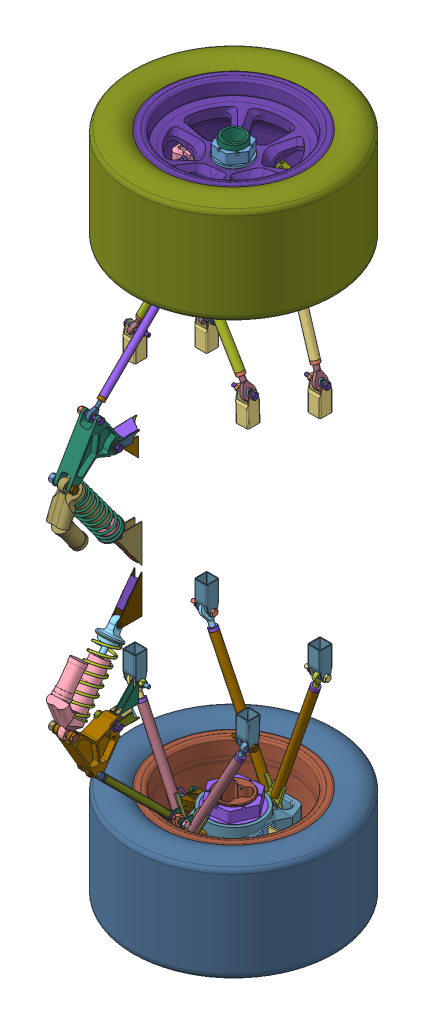
SolidWorks assembly UN-A1001-AB-Rear Unsprung Assembly, configuration Default. Lengths in mm. (continued)
Components (placement in the parent): (continued)
- SP-A0200-AH-Rear Axle AssemblyMirror-2: SP-A0200-AH-Rear Axle AssemblyMirror [Default] x (1 0 0) z (0 0 -1) size (274.88 563.57 484.64)
  - SP-AA-Rear Lower A-ArmMirror^SP-A0200-AH-Rear Axle Assembly-1: SP-AA-Rear Lower A-ArmMirror^SP-A0200-AH-Rear Axle Assembly [Default] at (0 -0.399 -0.6588) x (1 0 0) z (0 -0.002866 0.999996) size (222.76 290.57 36.42)
    - SP-Lower Apex RearMirror-1: SP-Lower Apex RearMirror [Default] at (-792.4265 549.6462 -121.5417) x (-0.932505 -0.360479 -0.022123) z (0 0.061256 -0.998122) size (54.94 63.8 9.53)
    - MirrorFS-MALE ROD END UNF-3A, 0.3125x24-0.25D (XAM-4)1Mirror-1: MirrorFS-MALE ROD END UNF-3A, 0.3125x24-0.25D (XAM-4)1Mirror [Default] at (-906.7265 255.0788 -139.6197) x (0.932505 -0.360479 -0.022123) z (0.361157 0.930754 0.057121)
    - MirrorFS-MALE ROD END UNF-3A, 0.3125x24-0.25D (XAM-4)1Mirror-2: MirrorFS-MALE ROD END UNF-3A, 0.3125x24-0.25D (XAM-4)1Mirror [Default] at (-678.1265 255.0788 -139.6197) x (0.932505 0.360479 0.022123) z (-0.361157 0.930754 0.057121)
    - SP-10003-AB-Threaded InsertMirror-1: SP-10003-AB-Threaded InsertMirror [A-Arm] at (-890.6731 296.4508 -137.0806) x (0.932505 -0.360479 -0.022123) z (0.361157 0.930754 0.057121) size (15.88 15.88 15.88)
    - SP-10003-AB-Threaded InsertMirror-2: SP-10003-AB-Threaded InsertMirror [A-Arm] at (-694.18 296.4508 -137.0806) x (0.932505 0.360479 0.022123) z (-0.361157 0.930754 0.057121) size (15.88 15.88 15.88)
    - SP-Rear Lower A-Arm TubeMirror-1: SP-Rear Lower A-Arm TubeMirror [Default] at (-838.6322 430.5677 -128.8497) x (-0.361157 -0.930754 -0.057121) z (0 0.061256 -0.998122) size (257.84 15.88 15.88)
    - SP-Rear Lower A-Arm TubeMirror-2: SP-Rear Lower A-Arm TubeMirror [Default] at (-746.2209 430.5677 -128.8497) x (0.361157 -0.930754 -0.057121) z (0 -0.061256 0.998122) size (257.84 15.88 15.88)
    - FS-HIGH MISALIGN SPHERICAL BEARING, 0.375-0.906D (3072-6G)Mirror-1: Assem24 [Default] at (-792.4265 549.6462 -121.5417) x (-0.932505 0.360479 0.022123) z (0.361157 0.930754 0.057121) size (26.46 21.71 26.13)
      - RaceMirror^FS-HIGH MISALIGN SPHERICAL BEARING, 0.375-0.906D (3072-6G)-1: Part65 [Default] at origin size (23.01 8.76 23.01)
      - BallMirror^FS-HIGH MISALIGN SPHERICAL BEARING, 0.375-0.906D (3072-6G)-1: Part66 [Default] x (0.359576 -0.008176 -0.93308) z (0.932238 0.046516 0.358844) size (19.84 20.65 19.84)
  - SP-AA-Rear Upper A-ArmMirror^SP-A0200-AH-Rear Axle Assembly-1: SP-AA-Rear Upper A-ArmMirror^SP-A0200-AH-Rear Axle Assembly [Default] at (-38.1 -1.9308 -1.9372) x (1 0 0) z (0 -0.00685 0.999977) size (216 215.55 29.43)
    - SP-Upper Apex RearMirror-1: SP-Upper Apex RearMirror [Default] at (-755.8405 523.8827 -293.8505) x (0.884705 -0.465567 0.023329) z (0 0.050046 0.998747) size (76.45 83.12 9.53)
    - MirrorFS-MALE ROD END UNF-3A, 0.3125x24-0.25D (XAM-4)1Mirror-1: MirrorFS-MALE ROD END UNF-3A, 0.3125x24-0.25D (XAM-4)1Mirror [Default] at (-870.1405 307.2255 -282.9942) x (0.884705 -0.465567 0.023329) z (0.466151 0.883596 -0.044276)
    - MirrorFS-MALE ROD END UNF-3A, 0.3125x24-0.25D (XAM-4)1Mirror-2: MirrorFS-MALE ROD END UNF-3A, 0.3125x24-0.25D (XAM-4)1Mirror [Default] at (-641.5405 307.2255 -282.9942) x (0.884705 0.465567 -0.023329) z (-0.466151 0.883596 -0.044276)
    - SP-10003-AB-Threaded InsertMirror-1: SP-10003-AB-Threaded InsertMirror [A-Arm] at (-849.4201 346.5014 -284.9623) x (0.884705 -0.465567 0.023329) z (0.466151 0.883596 -0.044276) size (15.88 15.88 15.88)
    - SP-10003-AB-Threaded InsertMirror-2: SP-10003-AB-Threaded InsertMirror [A-Arm] at (-662.261 346.5014 -284.9623) x (0.884705 0.465567 -0.023329) z (-0.466151 0.883596 -0.044276) size (15.88 15.88 15.88)
    - SP-Rear Upper A-Arm TubeMirror-1: SP-Rear Upper A-Arm TubeMirror [Default] at (-812.9905 415.5541 -288.4224) x (0.466151 0.883596 -0.044276) z (-0.884705 0.465567 -0.023329) size (186.28 15.88 15.88)
    - SP-Rear Upper A-Arm TubeMirror-2: SP-Rear Upper A-Arm TubeMirror [Default] at (-698.6905 415.5541 -288.4224) x (-0.466151 0.883596 -0.044276) z (-0.884705 -0.465567 0.023329) size (186.28 15.88 15.88)
    - FS-HIGH MISALIGN SPHERICAL BEARING, 0.375-0.906D (3072-6G)Mirror-1: Assem28 [Default] at (-755.8405 523.8827 -293.8505) x (0.884705 -0.465567 0.023329) z (0.466151 0.883596 -0.044276) size (26.46 21.71 26.13)
      - RaceMirror^FS-HIGH MISALIGN SPHERICAL BEARING, 0.375-0.906D (3072-6G)-1: Part69 [Default] at origin size (23.01 8.76 23.01)
      - BallMirror^FS-HIGH MISALIGN SPHERICAL BEARING, 0.375-0.906D (3072-6G)-1: Part70 [Default] x (0.359576 -0.008176 -0.93308) z (0.932238 0.046516 0.358844) size (19.84 20.65 19.84)
  - Assem8Mirror^SP-A0200-AH-Rear Axle Assembly-1: Assem8Mirror^SP-A0200-AH-Rear Axle Assembly [Default] at (-1592.9214 814.7933 -712.2762) x (-0.999891 -0.01037 -0.010464) z (-0.012143 0.982316 0.186836) size (17.98 166.51 230.13)
    - Part2Mirror^Assem8_SP-A0200-AH-Rear Axle Assembly-1: Part2Mirror^Assem8_SP-A0200-AH-Rear Axle Assembly [Default] at origin size (15.39 113.92 157.78)
    - SP-10003-AC-Threaded InsertMirror-1: SP-10003-AC-Threaded InsertMirror [AM-4 Rod End Thread] at (-799.064 427.6015 -294.0449) x (-0.999891 -0.008342 -0.012143) z (0.014733 -0.566176 -0.824153) size (12.7 12.7 15.88)
    - SP-10003-AC-Threaded InsertMirror-2: SP-10003-AC-Threaded InsertMirror [AM-4 Rod End Thread] at (-796.6527 334.9355 -428.9338) x (-0.999891 -0.008342 -0.012143) z (-0.014733 0.566176 0.824153) size (12.7 12.7 15.88)
    - FS-MALE ROD END UNF-3A, 0.25x28-0.25D (AM-4)Mirror-1: Assem30 [Default] at (-796.0446 311.5665 -462.9507) x (0 -0.824242 0.566238) z (0.014733 -0.566176 -0.824153) size (19.32 14.06 49.44)
      - BodyMirror^FS-MALE ROD END UNF-3A, 0.25x28-0.25D (AM-4)-1: Part73 [Default] at origin size (19.32 7.2 49.44)
      - BallMirror^FS-MALE ROD END UNF-3A, 0.25x28-0.25D (AM-4)-1: Part74 [Default] x (0.09633 0.218783 -0.971007) z (0.984027 -0.167661 0.059845) size (12.7 9.53 12.7)
    - FS-MALE ROD END UNF-3A, 0.25x28-0.25D (AM-4)Mirror-2: Assem31 [Default] at (-799.6721 450.9704 -260.028) x (0 -0.824242 0.566238) z (-0.014733 0.566176 0.824153) size (19.32 14.06 49.44)
      - BodyMirror^FS-MALE ROD END UNF-3A, 0.25x28-0.25D (AM-4)-1: Part75 [Default] at origin size (19.32 7.2 49.44)
      - BallMirror^FS-MALE ROD END UNF-3A, 0.25x28-0.25D (AM-4)-1: Part76 [Default] x (0.09633 0.218783 -0.971007) z (0.984027 -0.167661 0.059845) size (12.7 9.53 12.7)
  - SP-A0105-AC-Ohlin TTX25 MKII, 200mmMirror-1: SP-A0105-AC-Ohlin TTX25 MKII, 200mmMirror [Default] at (-793.9406 216.4917 -537.8809) x (-1 0 0) z (0 -0.803503 0.5953) size (48.39 85.02 197.6)
    - Shock BodyMirror^SP-A0105-AC-Ohlin TTX25 MKII, 200mm-1: Shock BodyMirror^SP-A0105-AC-Ohlin TTX25 MKII, 200mm [Default] at origin size (40.76 80 131.7)
    - HeadMirror^SP-A0105-AC-Ohlin TTX25 MKII, 200mm-1: HeadMirror^SP-A0105-AC-Ohlin TTX25 MKII, 200mm [Default] at (0 0 174.6) size (46 46 119)
    - BallMirror^SP-A0105-AC-Ohlin TTX25 MKII, 200mm-1: BallMirror^SP-A0105-AC-Ohlin TTX25 MKII, 200mm [Default] at (0 0 174.6) x (-0.011681 0.107343 -0.994153) z (-0.993776 -0.111394 -0.000351) size (15 15 8)
    - BallMirror^SP-A0105-AC-Ohlin TTX25 MKII, 200mm-2: BallMirror^SP-A0105-AC-Ohlin TTX25 MKII, 200mm [Default] x (0.079523 -0.862756 0.499328) z (-0.965926 0.057074 0.252448) size (15 15 8)
    - SP-#####-AB-SpringMirror-1: SP-#####-AB-SpringMirror [Default] at (0 0 151.1) size (48.39 49.05 127.97)
  - FS-BALL BEARING, 0.25ID-0.75OD (60355K702)Mirror-1: Part81 [Default] at (-784.8125 243.84 -446.6415) x (0 -0.287121 -0.957894) z (1 0 0) size (19.05 19.05 7.14)
  - FS-BALL BEARING, 0.25ID-0.75OD (60355K702)Mirror-2: Part82 [Default] at (-803.0688 243.84 -446.6415) x (0 0.287121 0.957894) z (-1 0 0) size (19.05 19.05 7.14)
  - FS-CADMIUM PLATED C3 HEX, 0.25x28-1.65-0.469 (AN4-13A)Mirror-1: Part83 [Default] at (-796.8362 310.0391 -484.3789) x (-1 0 0) z (0 -0.868755 0.495242) size (46.28 12.9 11.18)
  - FS-ZINC YELLOW CHROMATE C10.9 HX, M8x1.25-40-22 (95327A569)Mirror-1: Part84 [Default] at (-795.4156 216.4917 -537.8809) x (-1 0 0) z (0 0.287121 0.957894) size (45.3 15.01 13)
  - FS-NYLOC FLHX C8, M8x1.25-11.1 (92461A400)Mirror-1: Part85 [Default] at (-820.9156 216.4917 -537.8809) x (0 0.868058 0.496463) z (1 0 0) size (17.9 17.9 11.1)
  - FS-NYLOC G8 HX, 0.25x28-0.3125 (90630A145)Mirror-1: Part86 [Default] at (-809.8156 310.0391 -484.3789) x (0 0.868058 0.496463) z (0 -0.496463 0.868058) size (11.11 7.94 12.83)
  - SP-C30066-AA-A-Arm Tab BoxMirror-1: SP-C30066-AA-A-Arm Tab BoxMirror [Default] at (-680.9758 289.7175 -282.8202) x (-0.029021 0.999579 0) z (0 0 -1) size (60.32 25.4 25.4)
  - SP-C30066-AA-A-Arm Tab BoxMirror-2: SP-C30066-AA-A-Arm Tab BoxMirror [Default] at (-908.2405 289.7636 -282.8202) x (0 1 0) z (0 0 -1) size (60.32 25.4 25.4)
  - SP-C30066-AA-A-Arm Tab BoxMirror-3: SP-C30066-AA-A-Arm Tab BoxMirror [Default] at (-678.1265 237.6164 -139.5469) x (0 1 0) z (0 0 1) size (60.32 25.4 25.4)
  - SP-C30066-AA-A-Arm Tab BoxMirror-4: SP-C30066-AA-A-Arm Tab BoxMirror [Default] at (-906.7265 237.6164 -139.5469) x (0 1 0) z (0 0 1) size (60.32 25.4 25.4)
  - MirrorSP-30063-AB-Pushrod TabMirror-1: MirrorSP-30063-AB-Pushrod TabMirror [Default] at (-782.0343 483.2134 -293.6084) x (1 0 0) z (0 -0.043203 -0.999066) size (1.59 15.88 23.81)
  - MirrorSP-30063-AB-Pushrod TabMirror-2: MirrorSP-30063-AB-Pushrod TabMirror [Default] at (-805.8468 483.2134 -293.6084) x (-1 0 0) z (0 -0.043203 -0.999066) size (1.59 15.88 23.81)
  - FS-NYLOC FLHX C8, M8x1.25-11.1 (92461A400)Mirror-2: Part89 [Default] at (-820.9156 243.84 -446.6415) x (0 0 1) z (1 0 0) size (17.9 17.9 11.1)
  - FS-CADMIUM PLATED C3 HEX, 0.25x28-1.65-0.469 (AN4-13A)Mirror-2: Part90 [Default] at (-796.8362 243.84 -446.6415) x (-1 0 0) z (0 -0.287121 -0.957894) size (46.28 12.9 11.18)
  - FS-CADMIUM PLATED C3 HEX, 0.25x28-1.65-0.469 (AN4-13A)Mirror-3: Part91 [Default] at (-687.5506 306.9965 -282.8202) x (-0.999579 -0.029021 0) z (0 0 -1) size (46.28 12.9 11.18)
  - FS-CADMIUM PLATED C3 HEX, 0.25x28-1.65-0.469 (AN4-13A)Mirror-4: Part92 [Default] at (-902.1699 307.2261 -282.8202) size (46.28 12.9 11.18)
  - FS-CADMIUM PLATED C3 HEX, 0.25x28-1.65-0.469 (AN4-13A)Mirror-5: Part93 [Default] at (-912.7971 255.0789 -139.5469) x (-1 0 0) z (0 0 -1) size (46.28 12.9 11.18)
  - FS-CADMIUM PLATED C3 HEX, 0.25x28-1.65-0.469 (AN4-13A)Mirror-6: Part94 [Default] at (-684.1971 255.0789 -139.5469) x (-1 0 0) z (0 0 -1) size (46.28 12.9 11.18)
  - FS-CADMIUM PLATED C3 HEX, 0.25x28-1.65-0.469 (AN4-13A)Mirror-7: Part95 [Default] at (-799.2174 482.5275 -309.4686) x (-1 0 0) z (0 0.609051 0.793131) size (46.28 12.9 11.18)
  - FS-NYLOC G8 HX, 0.25x28-0.3125 (90630A145)Mirror-2: Part96 [Default] at (-807.4343 482.5275 -309.4686) x (0 -0.043203 -0.999066) z (0 0.999066 -0.043203) size (11.11 7.94 12.83)
  - FS-NYLOC G8 HX, 0.25x28-0.3125 (90630A145)Mirror-3: Part97 [Default] at (-694.1772 306.8041 -282.8202) x (-0.029021 0.999579 0) z (0 0 1) size (11.11 7.94 12.83)
  - FS-NYLOC G8 HX, 0.25x28-0.3125 (90630A145)Mirror-4: Part98 [Default] at (-895.5405 307.2261 -282.8202) x (0 1 0) z (0 0 -1) size (11.11 7.94 12.83)
  - FS-NYLOC G8 HX, 0.25x28-0.3125 (90630A145)Mirror-5: Part99 [Default] at (-919.4265 255.0789 -139.5469) x (0 1 0) z (0 0 1) size (11.11 7.94 12.83)
  - FS-NYLOC G8 HX, 0.25x28-0.3125 (90630A145)Mirror-6: Part100 [Default] at (-690.8265 255.0789 -139.5469) x (0 -1 0) z (0 0 -1) size (11.11 7.94 12.83)
  - FS-ROD END RETAINING WASHER, 0.25-0.245 (NO PN)Mirror-1: Part101 [Default] at (-781.9073 482.5275 -309.4686) x (0 1 0) z (1 0 0) size (12.7 12.7 6.22)
  - FS-ROD END RETAINING WASHER, 0.25-0.245 (NO PN)Mirror-2: Part102 [Default] at (-805.9738 482.5275 -309.4686) x (0 0.978954 -0.204082) z (-1 0 0) size (12.7 12.7 6.22)
  - SP-A0200-Rear Inner Rocker GussetMirror-1: SP-A0200-Rear Inner Rocker GussetMirror [Default] at (-793.9406 234.6955 -425.4808) x (1 0 0) z (0 -0.052336 0.99863) size (26.99 1.59 48.67)
  - SP-A0200-Rear Long Rocker TabMirror-1: SP-A0200-Rear Long Rocker TabMirror [Rear] at (-807.4344 243.84 -446.6415) x (1 0 0) z (0 0.00621 -0.999981) size (1.59 19.05 73.11)
  - SP-A0200-Rear Outer Rocker GussetMirror-1: SP-A0200-Rear Outer Rocker GussetMirror [Default] at (-793.9406 251.3902 -418.9606) x (1 0 0) z (0 0.039929 0.999203) size (26.99 1.59 43.52)
  - SP-A0200-Rear Rocker Gusset SupportMirror-1: SP-A0200-Rear Rocker Gusset SupportMirror [Default] at (-800.2906 228.5949 -403.7833) x (0 0 -1) z (0 -1 0) size (38.05 1.59 40.09)
  - SP-A0200-Rear Short Rocker TabMirror-1: SP-A0200-Rear Short Rocker TabMirror [Rear] at (-780.4469 243.8408 -446.6212) x (1 0 0) z (0 0.00621 -0.999981) size (1.59 17.17 50.59)
  - SP-A0200-Rear Rocker Gusset SupportMirror-2: SP-A0200-Rear Rocker Gusset SupportMirror [Default] at (-789.8131 228.5949 -403.7833) x (0 0 -1) z (0 -1 0) size (38.05 1.59 40.09)
  - SP-A0200-Rear Shock GussetMirror-1: SP-A0200-Rear Shock GussetMirror [Default] at (-793.9406 34.3591 -413.4634) x (1 0 0) z (0 -0.809017 0.587785) size (14.29 1.59 50.8)
  - SP-A0200-Rear Shock TabMirror-1: SP-A0200-Rear Shock TabMirror [Rear] at (-786.7969 76.2 -433.9415) x (-1 0 0) z (0 0.809017 -0.587785) size (1.59 45.95 88.76)
  - SP-A0200-Rear Shock TabMirror-2: SP-A0200-Rear Shock TabMirror [Front] at (-801.0844 76.2 -433.9415) x (-1 0 0) z (0 0.809017 -0.587785) size (1.59 45.95 88.76)
  - FS-MALE ROD END UNJF-3A, 0.375x24-0.25D (HXAM-4T)Mirror-1: Assem33 [Default] at (-679.6405 307.2261 -282.8202) x (0 0.043203 0.999066) z (0.466151 -0.883879 0.038222) size (26.22 15.06 62.54)
    - BodyMirror^FS-MALE ROD END UNJF-3A, 0.375x24-0.25D (HXAM-4T)-1: Part110 [no_threads] at origin size (26.22 9.62 62.54)
    - BallMirror^FS-MALE ROD END UNJF-3A, 0.375x24-0.25D (HXAM-4T)-1: Part111 [Default] at origin size (15.06 15.06 15.06)
  - FS-MALE ROD END UNJF-3A, 0.375x24-0.25D (HXAM-4T)Mirror-2: Assem34 [Default] at (-908.2405 307.2261 -282.8202) x (0 -0.043203 -0.999066) z (-0.466151 -0.883879 0.038222) size (26.22 15.06 62.54)
    - BodyMirror^FS-MALE ROD END UNJF-3A, 0.375x24-0.25D (HXAM-4T)-1: Part112 [no_threads] at origin size (26.22 9.62 62.54)
    - BallMirror^FS-MALE ROD END UNJF-3A, 0.375x24-0.25D (HXAM-4T)-1: Part113 [Default] at origin size (15.06 15.06 15.06)
  - FS-MALE ROD END UNJF-3A, 0.375x24-0.25D (HXAM-4T)Mirror-3: Assem35 [Default] at (-906.7265 255.0789 -139.5469) x (0 0.064116 -0.997942) z (-0.361157 -0.930586 -0.059789) size (26.22 15.06 62.54)
    - BodyMirror^FS-MALE ROD END UNJF-3A, 0.375x24-0.25D (HXAM-4T)-1: Part114 [no_threads] at origin size (26.22 9.62 62.54)
    - BallMirror^FS-MALE ROD END UNJF-3A, 0.375x24-0.25D (HXAM-4T)-1: Part115 [Default] at origin size (15.06 15.06 15.06)
  - FS-MALE ROD END UNJF-3A, 0.375x24-0.25D (HXAM-4T)Mirror-4: Assem36 [Default] at (-678.1265 255.0789 -139.5469) x (0 -0.064116 0.997942) z (0.361157 -0.930586 -0.059789) size (26.22 15.06 62.54)
    - BodyMirror^FS-MALE ROD END UNJF-3A, 0.375x24-0.25D (HXAM-4T)-1: Part116 [no_threads] at origin size (26.22 9.62 62.54)
    - BallMirror^FS-MALE ROD END UNJF-3A, 0.375x24-0.25D (HXAM-4T)-1: Part117 [Default] at origin size (15.06 15.06 15.06)
  - SP-B0100-Rear RockerMirror-1: SP-B0100-Rear RockerMirror [Default] at (14.7593 458.8134 310.4211) x (0.993764 -0.111506 0.000215) z (0.085107 0.759728 0.644647) size (43.51 92.41 122.03)
- WT-A0100-XG-Corner AssemblyMirror-2: WT-A0100-XG-Corner AssemblyMirror [Default] x (1 0 0) z (0 0 -1) size (411.48 213.6 411.53)
  - WT-00202-AA-Hoosier R25B 16x7_5-10Mirror-1: WT-00202-AA-Hoosier R25B 16x7_5-10Mirror [Default] at (-793.1174 574.9879 -198.909) x (-1 0 0) z (0 1 0.000253) size (411.48 411.48 213.5)
  - WT-00201-AA-OZ Centerlock 10in WheelMirror-1: WT-00201-AA-OZ Centerlock 10in WheelMirror [Default] at (-793.1174 596.9879 -198.9034) x (-0.992442 0.000031 -0.122714) z (0 -1 -0.000253) size (288.79 288.79 189.86)
  - WT-10105-AA-Drive PinMirror-1: WT-10105-AA-Drive PinMirror [Default] at (-825.0424 596.994 -223.0032) x (-0.121576 0.000251 -0.992582) z (0.992582 0.000031 -0.121576) size (12.67 23.01 11.95)
  - WT-10102-AA-Centerlock NutMirror-1: WT-10102-AA-Centerlock NutMirror [Default] at (-793.1174 647.6073 -198.8906) x (-0.440541 -0.000227 0.897732) z (-0.897733 0.000111 -0.440541) size (66 31.75 66)
  - WT-XF-UprightMirror-1: WT-XF-UprightMirror [Default] at (-793.1174 537.8923 -198.9183) x (-0.999961 -0.000002 0.008824) z (0.008824 -0.000253 0.999961) size (134.42 50.23 211.08)
  - BR-A0102-AA-Caliper AssemblyMirror-1: BR-A0102-AA-Caliper AssemblyMirror [Default] at (-874.0145 570.8565 -194.5235) x (-0.069854 0.000252 -0.997557) z (0 1 0.000253) size (82.63 68.94 66.64)
    - cp3838-M08x1.25m_CP4477-110Mirror^BR-A0102-AA-Caliper Assembly-1: Part124 [Default] at (-13.37 19.3 -19.55) x (-0.999952 -0.009843 0) z (0 0 -1) size (13 13 46)
    - CP4226-102Mirror^BR-A0102-AA-Caliper Assembly-1: CP4226-102Mirror^BR-A0102-AA-Caliper Assembly [Default] x (-1 0 0) z (0 0 -1) size (63.87 47.42 31.57)
    - cp4226-104_CP4226-104Mirror^BR-A0102-AA-Caliper Assembly-1: cp4226-104_CP4226-104Mirror^BR-A0102-AA-Caliper Assembly [Default] at (0 23 31.9644) x (0 0 -1) z (1 0 0) size (61.35 20.1 3)
    - CP4226-101Mirror^BR-A0102-AA-Caliper Assembly-1: CP4226-101Mirror^BR-A0102-AA-Caliper Assembly [Default] at origin size (81.26 55.69 34.68)
    - cp3838-M08x1.25m_CP4477-110Mirror^BR-A0102-AA-Caliper Assembly-2: Part128 [Default] at (13.37 19.3 -19.55) x (-0.997666 -0.068288 0) z (0 0 -1) size (13 13 46)
    - cp3049-40a_CP4226-103Mirror^BR-A0102-AA-Caliper Assembly-1: cp3049-40a_CP4226-103Mirror^BR-A0102-AA-Caliper Assembly [Default] at (0 0 -10.305) x (-0.993137 0.116957 0) z (0 0 -1) size (25.2 25.2 14.87)
    - CP4469-101Mirror^BR-A0102-AA-Caliper Assembly-1: CP4469-101Mirror^BR-A0102-AA-Caliper Assembly [Default] at (42 -11.5 23.98) x (0 -0.520643 -0.853775) z (1 0 0) size (9.18 8.2 29.15)
    - cp3049-40a_CP4226-103Mirror^BR-A0102-AA-Caliper Assembly-2: cp3049-40a_CP4226-103Mirror^BR-A0102-AA-Caliper Assembly [Default] at (0 0 10.305) size (25.2 25.2 14.87)
    - Brake PadMirror^BR-A0102-AA-Caliper Assembly-1: Brake PadMirror^BR-A0102-AA-Caliper Assembly [Default] at (0 11.1798 -8.5855) x (-1 0 0) z (0 1 0) size (39.62 6.86 43.54)
    - Brake PadMirror^BR-A0102-AA-Caliper Assembly-2: Brake PadMirror^BR-A0102-AA-Caliper Assembly [Default] at (0 11.1798 8.5905) x (1 0 0) z (0 1 0) size (39.62 6.86 43.54)
  - WT-10103-AA-Grease SealMirror-1: WT-10103-AA-Grease SealMirror [Default] at (-793.1174 559.091 -198.913) x (-0.781145 -0.000158 0.624349) z (0.624349 -0.000198 0.781145) size (97.66 13.92 97.66)
  - LL713049-LL713010-TheTimkenCompany-3D-11-03-2022.stpMirror-1: Part133 [Default] at (-793.1174 541.0673 -198.9175) x (0 1 0.000253) z (-0.586717 0.000205 -0.809792) size (15.53 98.42 98.42)
  - LL713049-LL713010-TheTimkenCompany-3D-11-03-2022.stpMirror-2: Part134 [Default] at (-793.1174 534.7173 -198.9191) x (0 -1 -0.000253) z (-0.531557 0.000214 -0.847022) size (15.53 98.42 98.42)
  - WT-XA-Tripod NutMirror-1: WT-XA-Tripod NutMirror [Default] at (-793.1174 516.4598 -198.9238) x (0 1 0.000253) z (-0.798123 0.000152 -0.602494) size (30.44 98.37 98.37)
  - WT-BA-Camber BlockMirror-1: WT-BA-Camber BlockMirror [Default] at (-793.95 547.3609 -293.2547) x (-0.999961 -0.000002 0.008824) z (0.008819 0.034647 0.999361) size (82.61 35.93 35.38)
  - 91290A442_Alloy Steel Socket Head ScrewMirror-1: 91290A442_Alloy Steel Socket Head ScrewMirror [91290A442] at (-816.177 556.8302 -293.3869) x (0.914102 0.014329 0.405231) z (-0.000308 0.9994 -0.034645) size (13 13 48.09)
  - BR-A0000-AB-Rear Brake AssemblyMirror-1: BR-A0000-AB-Rear Brake AssemblyMirror [Default] at (-793.1174 596.9879 -198.9034) x (-0.602494 -0.000202 0.798123) z (0.798123 -0.000152 0.602494) size (251.55 172.72 251.55)
    - WT-XA-#####-Tripod HubMirror-1: WT-XA-#####-Tripod HubMirror [Default] at origin size (102.86 172.72 102.86)
    - BR-20601-AB-Brake RotorMirror-1: BR-20601-AB-Brake RotorMirror [Default] at (0 26.1303 0) x (0.866025 0 0.5) z (-0.5 0 0.866025) size (184.15 4.76 184.15)
    - BR-20603-BA-Floating BobbinsMirror-1: BR-20603-BA-Floating BobbinsMirror [Default] at (39.8696 25.9874 -23.0188) size (15.88 8.92 15.88)
    - BR-20603-BA-Floating BobbinsMirror-2: BR-20603-BA-Floating BobbinsMirror [Default] at (0 25.9874 -46.0375) x (0.5 0 -0.866025) z (0.866025 0 0.5) size (15.88 8.92 15.88)
    - BR-20603-BA-Floating BobbinsMirror-3: BR-20603-BA-Floating BobbinsMirror [Default] at (-39.8696 25.9874 -23.0188) x (-0.5 0 -0.866025) z (0.866025 0 -0.5) size (15.88 8.92 15.88)
    - BR-20603-BA-Floating BobbinsMirror-4: BR-20603-BA-Floating BobbinsMirror [Default] at (-39.8696 25.9874 23.0188) x (-1 0 0) z (0 0 -1) size (15.88 8.92 15.88)
    - BR-20603-BA-Floating BobbinsMirror-5: BR-20603-BA-Floating BobbinsMirror [Default] at (0 25.9874 46.0375) x (-0.5 0 0.866025) z (-0.866025 0 -0.5) size (15.88 8.92 15.88)
    - BR-20603-BA-Floating BobbinsMirror-6: BR-20603-BA-Floating BobbinsMirror [Default] at (39.8696 25.9874 23.0188) x (0.5 0 0.866025) z (-0.866025 0 0.5) size (15.88 8.92 15.88)
    - WT-20104-AB-Rear Sensor RingMirror-1: WT-20104-AB-Rear Sensor RingMirror [Default] at (0 30.099 0) x (-0.882948 0 -0.469472) z (0 1 0) size (137 137 1.59)
    - 91590A121_External Retaining RingMirror-1: 91590A121_External Retaining RingMirror [91590A121] at (-39.8696 29.2354 -23.0188) x (0 1 0) z (0.857167 0 0.515038) size (0.64 14.63 13.25)
    - 91590A121_External Retaining RingMirror-2: 91590A121_External Retaining RingMirror [91590A121] at (-39.8696 29.2354 23.0188) x (0 1 0) z (0.87462 0 -0.48481) size (0.64 14.63 13.25)
    - 91590A121_External Retaining RingMirror-3: 91590A121_External Retaining RingMirror [91590A121] at (0 29.2354 46.0375) x (0 1 0) z (0.017452 0 -0.999848) size (0.64 14.63 13.25)
    - 91590A121_External Retaining RingMirror-4: 91590A121_External Retaining RingMirror [91590A121] at (39.8696 29.2354 23.0188) x (0 1 0) z (-0.857167 0 -0.515038) size (0.64 14.63 13.25)
    - 91590A121_External Retaining RingMirror-5: 91590A121_External Retaining RingMirror [91590A121] at (39.8696 29.2354 -23.0188) x (0 1 0) z (-0.87462 0 0.48481) size (0.64 14.63 13.25)
    - 91590A121_External Retaining RingMirror-6: 91590A121_External Retaining RingMirror [91590A121] at (0 29.2354 -46.0375) x (0 1 0) z (-0.017452 0 0.999848) size (0.64 14.63 13.25)
    - 97447A110_Aluminum Blind Rivets with Aluminum MandrelMirror-1: 97447A110_Aluminum Blind Rivets with Aluminum MandrelMirror [97447A110] at (9.6137 30.099 -51.8707) x (-0.302097 0 0.953277) z (0 -1 0) size (5.03 5.03 11.56)
    - 97447A110_Aluminum Blind Rivets with Aluminum MandrelMirror-2: 97447A110_Aluminum Blind Rivets with Aluminum MandrelMirror [97447A110] at (-40.1145 30.099 -34.261) x (0.674514 0 0.738262) z (0 -1 0) size (5.03 5.03 11.56)
    - 97447A110_Aluminum Blind Rivets with Aluminum MandrelMirror-3: 97447A110_Aluminum Blind Rivets with Aluminum MandrelMirror [97447A110] at (-49.7282 30.099 17.6097) x (0.976611 0 -0.215015) z (0 -1 0) size (5.03 5.03 11.56)
    - 97447A110_Aluminum Blind Rivets with Aluminum MandrelMirror-4: 97447A110_Aluminum Blind Rivets with Aluminum MandrelMirror [97447A110] at (-9.6137 30.099 51.8707) x (0.302097 0 -0.953277) z (0 -1 0) size (5.03 5.03 11.56)
    - 97447A110_Aluminum Blind Rivets with Aluminum MandrelMirror-5: 97447A110_Aluminum Blind Rivets with Aluminum MandrelMirror [97447A110] at (40.1145 30.099 34.261) x (-0.674514 0 -0.738262) z (0 -1 0) size (5.03 5.03 11.56)
    - 97447A110_Aluminum Blind Rivets with Aluminum MandrelMirror-6: 97447A110_Aluminum Blind Rivets with Aluminum MandrelMirror [97447A110] at (49.7282 30.099 -17.6097) x (-0.976611 0 0.215015) z (0 -1 0) size (5.03 5.03 11.56)
  - FS-Jet Nut, M8x1.25 (MJET-M8X1.25)Mirror-1: Part144 [Default] at (-816.1783 561.0546 -293.5333) x (-0.906747 0.01433 0.421432) z (0.000308 -0.9994 0.034645) size (13.6 13.6 7)
  - 91290A442_Alloy Steel Socket Head ScrewMirror-2: 91290A442_Alloy Steel Socket Head ScrewMirror [91290A442] at (-771.7287 556.8303 -293.7791) x (-0.549228 0.028783 0.835176) z (-0.000308 0.9994 -0.034645) size (13 13 48.09)
  - FS-Jet Nut, M8x1.25 (MJET-M8X1.25)Mirror-2: Part145 [Default] at (-771.73 561.0547 -293.9256) x (0.139109 0.034351 0.989681) z (0.000308 -0.9994 0.034645) size (13.6 13.6 7)
  - WT-10105-AA-Drive PinMirror-2: WT-10105-AA-Drive PinMirror [Default] at (-769.0177 596.9959 -230.8283) x (0.992582 0.000031 -0.121576) z (0.121576 -0.000251 0.992582) size (12.67 23.01 11.95)
  - WT-10105-AA-Drive PinMirror-3: WT-10105-AA-Drive PinMirror [Default] at (-761.1925 596.9818 -174.8036) x (0.121576 -0.000251 0.992582) z (-0.992582 -0.000031 0.121576) size (12.67 23.01 11.95)
  - WT-10105-AA-Drive PinMirror-4: WT-10105-AA-Drive PinMirror [Default] at (-817.2172 596.9798 -166.9785) x (-0.992582 -0.000031 0.121576) z (-0.121576 0.000251 -0.992582) size (12.67 23.01 11.95)
  - WT-AA-#####-Rear Toe Backing PlateMirror-1: WT-AA-#####-Rear Toe Backing PlateMirror [Default] at (-737.6079 537.8924 -199.4082) x (0.999961 0.000002 -0.008824) z (0.008824 -0.000253 0.999961) size (3.17 25.4 50.8)
  - WT-AA-#####-Rear Toe Top ClevisMirror-1: WT-AA-#####-Rear Toe Top ClevisMirror [Default] at (-737.7085 541.0703 -210.8115) x (0.999961 0.000002 -0.008824) z (0.008824 -0.000253 0.999961) size (31.75 27.83 3.17)
  - WT-AA-#####-Rear Toe Bottom ClevisMirror-1: WT-AA-#####-Rear Toe Bottom ClevisMirror [Default] at (-737.4815 537.8888 -185.0832) x (0.999961 0.000002 -0.008824) z (0.008824 -0.000253 0.999961) size (31.75 27.12 3.17)
Mates (geometry in assembly coordinates):
- Coincident1: coincident: point of ?
- Coincident2: coincident: line of SP-A0200-AH-Rear Axle Assembly-1 through (307.2261 -793.9405 0) axis (0 0 1)
- Coincident3: coincident: line of SP-A0200-AH-Rear Axle Assembly-1 through (0 792.4265 0) axis (0 0 -1)
- Parallel1: parallel: line of SP-A0200-AH-Rear Axle Assembly-1 through (307.2261 -793.9405 0) axis (0 0 1)
- Parallel2: parallel: line of SP-A0200-AH-Rear Axle Assembly-1 through (0 792.4265 0) axis (0 0 -1)
- Coincident5: coincident: point of SP-A0200-AH-Rear Axle Assembly-1; point of WT-A0100-XG-Corner Assembly-1
- Coincident6: coincident aligned: line of SP-A0200-AH-Rear Axle Assembly-1 through (0 792.4265 0) axis (0 0 -1); line of WT-A0100-XG-Corner Assembly-1 through (0 792.4265 0) axis (0 0 -1)
- Coincident7: coincident aligned: line of SP-A0200-AH-Rear Axle Assembly-1 through (307.2261 -793.9405 0) axis (0 0 1); line of WT-A0100-XG-Corner Assembly-1 through (307.2261 -793.9405 0) axis (0 0 1)
